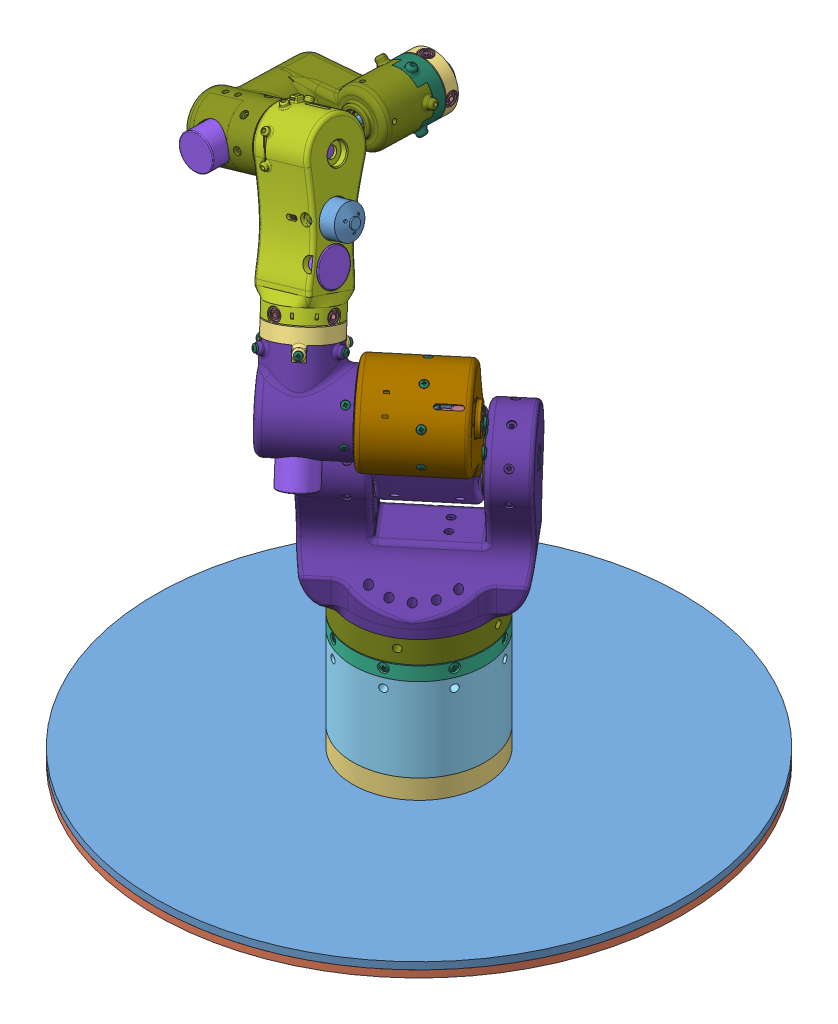
SolidWorks assembly Robotic Arm - Final Assembly, configuration Default. Lengths in mm.
Overall size (819.62 693.08 819.62).
163 component instances, 57 part files, 15 mates.
Components (placement in the parent):
- Bottom Base Assembly-1: Bottom Base Assembly [Default] at (29.9883 409.5515 787.0845) size (819.62 16 819.62)
  - Top Plate-1: Top Plate [Default] at origin size (600 8 600)
  - Bottom Plate-1: Bottom Plate [Default] at (0 -8 0) x (0.866025 0 -0.5) z (0.5 0 0.866025) size (600 8 600)
- A1 - Final Assembly-1: A1 - Final Assembly [Default] at (29.9883 417.5515 787.0845) x (0.866025 0 0.5) z (-0.5 0 0.866025) size (210.32 133.5 210.32)
  - A1D1 - Bottom-1: A1D1 - Bottom [Default] at origin size (150 22 150)
  - Turnigy Aerodrive SK3 4250-1: Turnigy Aerodrive SK3 4250 [Default] at (0 73.3 0) x (-0.707107 0 -0.707107) z (-0.707107 0 0.707107) size (52.1 79.08 41.8)
  - A1D2 - Middle-1: A1D2 - Middle [Default] at (0 22 0) x (0.991445 0 -0.130526) z (0.130526 0 0.991445) size (150 96 150)
  - A1D3 - Top-1: A1D3 - Top [Default] at (0 117 0) x (0.793353 0 0.608761) z (-0.608761 0 0.793353) size (150 15.5 150)
  - A1D4 - Encoder bracket-1: A1D4 - Encoder bracket [Default] at (0 30 0) x (0.991445 0 -0.130526) z (0.130526 0 0.991445) size (52.04 50 76.58)
  - Encoder600PR-1: Encoder600PR [Default] at (-40.4994 32.32 -24.4547) x (0.84353 0 0.537082) z (-0.537082 0 0.84353) size (38 53 38)
  - A1P1_S1 - BLDC Axis Bottom (50T HTD3m)-1: A1P1_S1 - BLDC Axis Bottom (50T HTD3m) [Default] at (-3.3955 88.2939 1.3517) x (0.767493 0 -0.641057) z (0 -1 0) size (46.98 46.92 14.7)
  - A1P1_S2 - BLDC Axis Top (Sun in A1R1)-1: A1P1_S2 - BLDC Axis Top (Sun in A1R1) [Default] at (-3.3955 88.2939 1.3517) x (0.767493 0 -0.641057) z (0 -1 0) size (38.1 38.1 28.24)
  - A1P2 - Encoder Axis (20T HTD3m)-1: A1P2 - Encoder Axis (20T HTD3m) [Default] at (-40.4994 73.3 -24.4547) x (0.825705 0 -0.564102) z (0 1 0) size (21.34 40.98 60.33)
  - radial ball bearing_68_am-3: radial ball bearing_68_am [AFBMA 20.1 - 00-70 - 18,DE,AC,18_68] at (0 126 0) x (0 1 0) z (0 0 1) size (13.2 110 110)
  - radial ball bearing_68_iso-1: radial ball bearing_68_iso [ISO 15 RBB - 105 - 8,SI,NC,8_68] at (8.4842 126.5 64.4439) x (0.130526 0 0.991445) z (-0.991445 0 0.130526) size (5 14 14)
  - radial ball bearing_68_iso-2: radial ball bearing_68_iso [ISO 15 RBB - 105 - 8,SI,NC,8_68] at (51.568 126.5 39.5695) x (0.793353 0 0.608761) z (-0.608761 0 0.793353) size (5 14 14)
  - radial ball bearing_68_iso-3: radial ball bearing_68_iso [ISO 15 RBB - 105 - 8,SI,NC,8_68] at (64.4439 126.5 -8.4842) x (0.991445 0 -0.130526) z (0.130526 0 0.991445) size (5 14 14)
  - radial ball bearing_68_iso-4: radial ball bearing_68_iso [ISO 15 RBB - 105 - 8,SI,NC,8_68] at (39.5695 126.5 -51.568) x (0.608761 0 -0.793353) z (0.793353 0 0.608761) size (5 14 14)
  - radial ball bearing_68_iso-5: radial ball bearing_68_iso [ISO 15 RBB - 105 - 8,SI,NC,8_68] at (-8.4842 126.5 -64.4439) x (-0.130526 0 -0.991445) z (0.991445 0 -0.130526) size (5 14 14)
  - radial ball bearing_68_iso-6: radial ball bearing_68_iso [ISO 15 RBB - 105 - 8,SI,NC,8_68] at (-51.568 126.5 -39.5695) x (-0.793353 0 -0.608761) z (0.608761 0 -0.793353) size (5 14 14)
  - radial ball bearing_68_iso-7: radial ball bearing_68_iso [ISO 15 RBB - 105 - 8,SI,NC,8_68] at (-64.4439 126.5 8.4842) x (-0.991445 0 0.130526) z (-0.130526 0 -0.991445) size (5 14 14)
  - radial ball bearing_68_iso-8: radial ball bearing_68_iso [ISO 15 RBB - 105 - 8,SI,NC,8_68] at (-39.5695 126.5 51.568) x (-0.608761 0 0.793353) z (-0.793353 0 -0.608761) size (5 14 14)
  - A1R1 - Fixed ring (38T)-1: A1R1 - Fixed ring (38T) [Default] at (-96.4762 151.2552 -44.9758) x (0.965926 0 0.258819) z (0 1 0) size (84.14 84.14 19.84)
  - pan head cross recess screw_iso-3: pan head cross recess screw_iso [ISO 7045 - M5 x 16 - Z - 16N] at (9.7764 126.5 74.2592) x (-0.130526 0 -0.991445) z (0.264332 -0.963804 -0.0348) size (19.63 9.5 9.5)
  - pan head cross recess screw_iso-5: pan head cross recess screw_iso [ISO 7045 - M4 x 16 - Z - 16N] at (6.8787 106.5867 52.2491) x (-0.130526 0 -0.991445) z (-0.096727 -0.995229 0.012734) size (19.02 8 8)
  - pan head cross recess screw_iso-6: pan head cross recess screw_iso [ISO 7045 - M4 x 16 - Z - 16N] at (30 128.5 51.9615) x (0 -1 0) z (0.614442 0 0.788962) size (19.02 8 8)
  - pan head cross recess screw_iso-7: pan head cross recess screw_iso [ISO 7045 - M4 x 16 - Z - 16N] at (41.8097 106.5867 32.0817) x (-0.793353 0 -0.608761) z (-0.059392 -0.995229 0.077401) size (19.02 8 8)
  - pan head cross recess screw_iso-8: pan head cross recess screw_iso [ISO 7045 - M4 x 16 - Z - 16N] at (52.2491 106.5867 -6.8787) x (-0.991445 0 0.130526) z (0.012734 -0.995229 0.096727) size (19.02 8 8)
  - pan head cross recess screw_iso-9: pan head cross recess screw_iso [ISO 7045 - M4 x 16 - Z - 16N] at (32.0817 106.5867 -41.8097) x (-0.608761 0 0.793353) z (0.077401 -0.995229 0.059392) size (19.02 8 8)
  - pan head cross recess screw_iso-10: pan head cross recess screw_iso [ISO 7045 - M4 x 16 - Z - 16N] at (-6.8787 106.5867 -52.2491) x (0.130526 0 0.991445) z (0.096727 -0.995229 -0.012734) size (19.02 8 8)
  - pan head cross recess screw_iso-11: pan head cross recess screw_iso [ISO 7045 - M4 x 16 - Z - 16N] at (-41.8097 106.5867 -32.0817) x (0.793353 0 0.608761) z (0.059392 -0.995229 -0.077401) size (19.02 8 8)
  - pan head cross recess screw_iso-12: pan head cross recess screw_iso [ISO 7045 - M4 x 16 - Z - 16N] at (-52.2491 106.5867 6.8787) x (0.991445 0 -0.130526) z (-0.012734 -0.995229 -0.096727) size (19.02 8 8)
  - pan head cross recess screw_iso-13: pan head cross recess screw_iso [ISO 7045 - M4 x 16 - Z - 16N] at (-32.0817 106.5867 41.8097) x (0.608761 0 -0.793353) z (-0.077401 -0.995229 -0.059392) size (19.02 8 8)
  - pan head cross recess screw_iso-14: pan head cross recess screw_iso [ISO 7045 - M4 x 16 - Z - 16N] at (57.9555 128.5 15.5291) x (0 -1 0) z (0.992357 0 0.123404) size (19.02 8 8)
  - pan head cross recess screw_iso-15: pan head cross recess screw_iso [ISO 7045 - M4 x 16 - Z - 16N] at (51.9615 128.5 -30) x (0 -1 0) z (0.788962 0 -0.614442) size (19.02 8 8)
  - pan head cross recess screw_iso-16: pan head cross recess screw_iso [ISO 7045 - M4 x 16 - Z - 16N] at (15.5291 128.5 -57.9555) x (0 -1 0) z (0.123404 0 -0.992357) size (19.02 8 8)
  - pan head cross recess screw_iso-17: pan head cross recess screw_iso [ISO 7045 - M4 x 16 - Z - 16N] at (-30 128.5 -51.9615) x (0 -1 0) z (-0.614442 0 -0.788962) size (19.02 8 8)
  - pan head cross recess screw_iso-18: pan head cross recess screw_iso [ISO 7045 - M4 x 16 - Z - 16N] at (-57.9555 128.5 -15.5291) x (0 -1 0) z (-0.992357 0 -0.123404) size (19.02 8 8)
  - pan head cross recess screw_iso-19: pan head cross recess screw_iso [ISO 7045 - M4 x 16 - Z - 16N] at (-51.9615 128.5 30) x (0 -1 0) z (-0.788962 0 0.614442) size (19.02 8 8)
  - pan head cross recess screw_iso-20: pan head cross recess screw_iso [ISO 7045 - M4 x 16 - Z - 16N] at (-15.5291 128.5 57.9555) x (0 -1 0) z (-0.123404 0 0.992357) size (19.02 8 8)
  - pan head cross recess screw_iso-21: pan head cross recess screw_iso [ISO 7045 - M5 x 16 - Z - 16N] at (59.4222 126.5 45.5962) x (-0.793353 0 -0.608761) z (0.162304 -0.963804 -0.211518) size (19.63 9.5 9.5)
  - pan head cross recess screw_iso-22: pan head cross recess screw_iso [ISO 7045 - M5 x 16 - Z - 16N] at (74.2592 126.5 -9.7764) x (-0.991445 0 0.130526) z (-0.0348 -0.963804 -0.264332) size (19.63 9.5 9.5)
  - pan head cross recess screw_iso-23: pan head cross recess screw_iso [ISO 7045 - M5 x 16 - Z - 16N] at (45.5962 126.5 -59.4222) x (-0.608761 0 0.793353) z (-0.211518 -0.963804 -0.162304) size (19.63 9.5 9.5)
  - pan head cross recess screw_iso-24: pan head cross recess screw_iso [ISO 7045 - M5 x 16 - Z - 16N] at (-9.7764 126.5 -74.2592) x (0.130526 0 0.991445) z (-0.264332 -0.963804 0.0348) size (19.63 9.5 9.5)
  - pan head cross recess screw_iso-25: pan head cross recess screw_iso [ISO 7045 - M5 x 16 - Z - 16N] at (-59.4222 126.5 -45.5962) x (0.793353 0 0.608761) z (-0.162304 -0.963804 0.211518) size (19.63 9.5 9.5)
  - pan head cross recess screw_iso-26: pan head cross recess screw_iso [ISO 7045 - M5 x 16 - Z - 16N] at (-74.2592 126.5 9.7764) x (0.991445 0 -0.130526) z (0.0348 -0.963804 0.264332) size (19.63 9.5 9.5)
  - pan head cross recess screw_iso-27: pan head cross recess screw_iso [ISO 7045 - M5 x 16 - Z - 16N] at (-45.5962 126.5 59.4222) x (0.608761 0 -0.793353) z (0.211518 -0.963804 0.162304) size (19.63 9.5 9.5)
  - pan head cross recess screw_iso-29: pan head cross recess screw_iso [ISO 7045 - M5 x 16 - Z - 16N] at (-75.73 69.5 20.0563) x (0.991445 0 -0.130526) z (-0.041237 0.948782 -0.313228) size (19.63 9.5 9.5)
  - pan head cross recess screw_iso-30: pan head cross recess screw_iso [ISO 7045 - M5 x 16 - Z - 16N] at (-78.3405 69.5 0.2274) x (0.991445 0 -0.130526) z (0.119155 0.408217 0.905075) size (19.63 9.5 9.5)
- A2 - Final Assembly-1: A2 - Final Assembly [Default] at (-49.7513 476.7623 907.6561) x (-0.868697 0 -0.495343) z (0.495343 0 -0.868697) size (219.53 224.2 242.26)
  - A2D1 - Bottom-1: A2D1 - Bottom [Default] at (-9.5453 74.2892 144.2387) size (150 26.12 150)
  - A2D2 - Top-1: A2D2 - Top [Default] at (-9.5453 109.2892 144.2387) x (0.347743 0 -0.93759) z (0.93759 0 0.347743) size (198.9 180.3 160.37)
  - A2D4 - Motor Bracket-1: A2D4 - Motor Bracket [Default] at (7.8419 132.7892 97.3592) x (-0.93759 0 -0.347743) z (0 -1 0) size (40 16 65)
  - A2D3 - Encoder Bracket-1: A2D3 - Encoder Bracket [Default] at (-16.8479 132.7892 163.9281) x (0.93759 0 0.347743) z (-0.347743 0 0.93759) size (40 41.5 8)
  - Turnigy Aerodrive SK3 4250-1: Turnigy Aerodrive SK3 4250 [Default] at (-9.9973 132.7892 145.4575) x (0.662976 -0.707107 0.245892) z (0.662976 0.707107 0.245892) size (52.1 79.08 41.8)
  - Encoder600PR-1: Encoder600PR [Default] at (-31.8008 132.7892 204.2444) x (0.468795 -0.866025 0.173872) z (0.811977 0.5 0.301155) size (38 53 38)
  - A2D5 - Motor To Encoder Connector-1: A2D5 - Motor To Encoder Connector [Default] at (-9.9973 132.7892 145.4575) x (0.662976 -0.707107 0.245892) z (-0.347743 0 0.93759) size (22 22 21.7)
  - A2R1 - Output Ring (36T)-1: A2R1 - Output Ring (36T) [Default] at (21.7427 110.9929 177.6385) x (0.683984 0 0.729497) z (0 1 0) size (82 82 36.22)
  - A2R2 - Fixed Ring (38T)-1: A2R2 - Fixed Ring (38T) [Default] at (6.8682 231.7999 101.2643) x (0.93759 0 0.347743) z (0.347743 0 -0.93759) size (77.7 77.7 19)
  - A2R2 - Fixed Ring (38T)-3: A2R2 - Fixed Ring (38T) [Default] at (-33.609 231.7999 207.84) x (-0.93759 0 -0.347743) z (-0.347743 0 0.93759) size (77.7 77.7 19)
  - radial ball bearing_68_iso-1: radial ball bearing_68_iso [ISO 15 RBB - 1860 - 32,SI,NC,32_68] at (4.0167 231.7892 107.6727) x (0.347743 0 -0.93759) z (0.369105 -0.91925 0.136897) size (10 78 78)
  - radial ball bearing_68_iso-2: radial ball bearing_68_iso [ISO 15 RBB - 1860 - 32,SI,NC,32_68] at (-30.7576 231.7892 201.4317) x (-0.347743 0 0.93759) z (-0.369105 0.91925 -0.136897) size (10 78 78)
  - radial ball bearing_68_din-1: radial ball bearing_68_din [DIN 625 - 608 - 8,DE,NC,8_68] at (22.9687 231.7892 56.574) x (0.347743 0 -0.93759) z (-0.181317 0.981123 -0.067249) size (7 22 22)
  - radial ball bearing_68_din-2: radial ball bearing_68_din [DIN 625 - 608 - 8,DE,NC,8_68] at (-42.0593 231.7892 231.9033) x (0.347743 0 -0.93759) z (0.862216 -0.392835 0.319788) size (7 22 22)
  - A2D8 Axis D8 220mm-1: A2D8 Axis D8 220mm [Default] at (24.1858 231.7892 53.2925) x (0.915947 -0.213623 0.339716) z (-0.347743 0 0.93759) size (8 8 194)
  - A2P1 - Motor and Axis-1: A2P1 - Motor and Axis [Default] at (17.5787 132.7892 71.1067) x (0.879075 0.347743 0.326041) z (0.326041 -0.93759 0.120925) size (21 22 21)
  - A2P1 - Motor and Axis-2: A2P1 - Motor and Axis [Default] at (12.7103 231.7892 84.2329) x (-0.937346 -0.02278 -0.347653) z (0.021358 -0.999741 0.007921) size (21 22 21)
- A3 - Final Assembly-1: A3 - Final Assembly [Default] at (19.335 680.5082 758.7988) x (-0.766512 0 0.64223) z (-0.450257 0.713079 -0.537389) size (116.5 270 98)
  - A3D1 - Bottom-1: A3D1 - Bottom [Default] at origin size (99.9 135 87.01)
  - A3D2 - Top-1: A3D2 - Top [Default] at (-94.5 331 0) x (0 1 0) z (-1 0 0) size (160 98 100.36)
  - A3D3 - Motor Assembly-1: A3D3 - Motor Assembly [Default] at (-19.5 149 0) x (0 0 1) z (0 -1 0) size (46 63 103.52)
  - Turnigy Aerodrive SK3 4250-1: Turnigy Aerodrive SK3 4250 [Default] at (31.8 149 0) x (0 -0.575127 0.818064) z (0 -0.818064 -0.575127) size (52.1 79.08 41.8)
  - Encoder600PR-1: Encoder600PR [Default] at (-19.5 107 0) x (0 -0.866025 0.5) z (0 0.5 0.866025) size (38 53 38)
  - A3D8 - Motor Assembly Gear 1-1: A3D8 - Motor Assembly Gear 1 [Default] at (71.5096 132.326 18.6577) x (1 0 0) z (0 0.420901 0.907106) size (4 42.98 42.98)
  - A3D9 - Motor Assembly Gear 2-1: A3D9 - Motor Assembly Gear 2 [Default] at (-13.5987 96.6456 14.6355) x (-1 0 0) z (0 -0.921751 -0.387782) size (15 43.41 43.41)
  - Pulley HTD_3mm T20 D5-1: Pulley HTD_3mm T20 D5 [Default] at (-41.5 149 0) x (0 -0.987714 0.156271) z (0 0.156271 0.987714) size (21 22 21)
  - A3D4 - Output Ring-1: A3D4 - Output Ring [Default] at (1.3 221.0108 0.045) x (0 0 -1) z (-1 0 0) size (76.49 77.19 18.96)
  - radial ball bearing_68_iso-1: radial ball bearing_68_iso [ISO 15 RBB - 1860 - 32,SI,NC,32_68] at (8.8 221 0) size (10 78 78)
  - radial ball bearing_68_iso-2: radial ball bearing_68_iso [ISO 15 RBB - 1860 - 32,SI,NC,32_68] at (42.5 221 0) x (1 0 0) z (0 -0.007607 0.999971) size (10 78 78)
  - Axis D8 197mm-1: Axis D8 197mm [Default] at (-52.5 221 0) x (0 0 -1) z (1 0 0) size (8 8 114)
  - radial ball bearing_68_din-1: radial ball bearing_68_din [DIN 625 - 608 - 8,DE,NC,8_68] at (-49 221 0) x (-1 0 0) z (0 -0.924225 -0.381849) size (7 22 22)
  - Pulley HTD_3mm T20 D5-3: Pulley HTD_3mm T20 D5 [Default] at (-41.5 221 0) x (0 0.38968 0.92095) z (0 0.92095 -0.38968) size (21 22 21)
  - A3D5 - Input Ring-1: A3D5 - Input Ring [Default] at (53.8 40 0) x (0 0 -1) z (1 0 0) size (65.4 65.4 34.7)
  - A3D5 - Input Ring-2: A3D5 - Input Ring [Default] at (-53.8 40 0) x (0 0 1) z (-1 0 0) size (65.4 65.4 34.7)
  - pan head cross recess screw_iso-3: pan head cross recess screw_iso [ISO 7045 - M4 x 16 - Z - 16N] at (-26.3 53.202 -36.2721) x (0 -0.34202 0.939693) z (-0.509751 -0.808438 -0.294247) size (19.02 8 8)
  - pan head cross recess screw_iso-4: pan head cross recess screw_iso [ISO 7045 - M4 x 16 - Z - 16N] at (-26.3 17.8599 -31.6193) x (0 0.573576 0.819152) z (-0.509751 -0.704734 0.49346) size (19.02 8 8)
  - pan head cross recess screw_iso-5: pan head cross recess screw_iso [ISO 7045 - M4 x 16 - Z - 16N] at (-26.3 1.4 0) x (0 1 0) z (-0.509751 0 0.860322) size (19.02 8 8)
  - pan head cross recess screw_iso-6: pan head cross recess screw_iso [ISO 7045 - M4 x 16 - Z - 16N] at (-26.3 17.8599 31.6193) x (0 0.573576 -0.819152) z (-0.509751 0.704734 0.49346) size (19.02 8 8)
  - pan head cross recess screw_iso-7: pan head cross recess screw_iso [ISO 7045 - M4 x 16 - Z - 16N] at (-26.3 53.202 36.2721) x (0 -0.34202 -0.939693) z (-0.509751 0.808438 -0.294247) size (19.02 8 8)
  - pan head cross recess screw_iso-12: pan head cross recess screw_iso [ISO 7045 - M4 x 16 - Z - 16N] at (26.2 53.202 36.2721) x (0 -0.34202 -0.939693) z (-0.509751 0.808438 -0.294247) size (19.02 8 8)
  - pan head cross recess screw_iso-13: pan head cross recess screw_iso [ISO 7045 - M4 x 16 - Z - 16N] at (26.2 17.8599 31.6193) x (0 0.573576 -0.819152) z (-0.509751 0.704734 0.49346) size (19.02 8 8)
  - pan head cross recess screw_iso-14: pan head cross recess screw_iso [ISO 7045 - M4 x 16 - Z - 16N] at (26.2 1.4 0) x (0 1 0) z (-0.509751 0 0.860322) size (19.02 8 8)
  - pan head cross recess screw_iso-15: pan head cross recess screw_iso [ISO 7045 - M4 x 16 - Z - 16N] at (26.2 17.8599 -31.6193) x (0 0.573576 0.819152) z (-0.509751 -0.704734 0.49346) size (19.02 8 8)
  - pan head cross recess screw_iso-16: pan head cross recess screw_iso [ISO 7045 - M4 x 16 - Z - 16N] at (26.2 53.202 -36.2721) x (0 -0.34202 0.939693) z (-0.509751 -0.808438 -0.294247) size (19.02 8 8)
  - pan head cross recess screw_iso-17: pan head cross recess screw_iso [ISO 7045 - M4 x 16 - Z - 16N] at (-7.2 201.8276 -46.2864) x (0 0.382683 0.92388) z (-0.246103 -0.895464 0.370913) size (19.02 8 8)
  - pan head cross recess screw_iso-18: pan head cross recess screw_iso [ISO 7045 - M4 x 16 - Z - 16N] at (-7.2 240.1724 -46.2864) x (0 -0.382683 0.92388) z (-0.246103 -0.895464 -0.370913) size (19.02 8 8)
  - pan head cross recess screw_iso-19: pan head cross recess screw_iso [ISO 7045 - M4 x 16 - Z - 16N] at (-7.2 267.2864 -19.1724) x (0 -0.92388 0.382683) z (-0.246103 -0.370913 -0.895464) size (19.02 8 8)
  - pan head cross recess screw_iso-20: pan head cross recess screw_iso [ISO 7045 - M4 x 16 - Z - 16N] at (-7.2 267.2864 19.1724) x (0 -0.92388 -0.382683) z (-0.246103 0.370913 -0.895464) size (19.02 8 8)
  - pan head cross recess screw_iso-21: pan head cross recess screw_iso [ISO 7045 - M4 x 16 - Z - 16N] at (-7.2 240.1724 46.2864) x (0 -0.382683 -0.92388) z (-0.246103 0.895464 -0.370913) size (19.02 8 8)
  - pan head cross recess screw_iso-22: pan head cross recess screw_iso [ISO 7045 - M4 x 16 - Z - 16N] at (-7.2 201.8276 46.2864) x (0 0.382683 -0.92388) z (-0.246103 0.895464 0.370913) size (19.02 8 8)
  - pan head cross recess screw_iso-23: pan head cross recess screw_iso [ISO 7045 - M4 x 16 - Z - 16N] at (50.6 128 14) x (-1 0 0) z (0 -0.78047 0.625193) size (19.02 8 8)
  - pan head cross recess screw_iso-24: pan head cross recess screw_iso [ISO 7045 - M4 x 16 - Z - 16N] at (50.6 128 -14) x (-1 0 0) z (0 -0.872039 0.489436) size (19.02 8 8)
  - pan head cross recess screw_iso-25: pan head cross recess screw_iso [ISO 7045 - M4 x 16 - Z - 16N] at (-6.6 178.2028 10) x (-1 0 0) z (0 -0.78047 0.625193) size (19.02 8 8)
  - pan head cross recess screw_iso-26: pan head cross recess screw_iso [ISO 7045 - M4 x 16 - Z - 16N] at (-6.6 178.2028 -10) x (-1 0 0) z (0 -0.857112 0.51513) size (19.02 8 8)
  - pan head cross recess screw_iso-28: pan head cross recess screw_iso [ISO 7045 - M5 x 20 - Z - 20N] at (-51.2 129.5 12) size (23.63 9.5 9.5)
  - pan head cross recess screw_iso-30: pan head cross recess screw_iso [ISO 7045 - M5 x 20 - Z - 20N] at (-51.2 129.5 -12) size (23.63 9.5 9.5)
  - pan head cross recess screw_iso-31: pan head cross recess screw_iso [ISO 7045 - M5 x 20 - Z - 20N] at (-48.9707 102 10) x (1 0 0) z (0 -0.0226 0.999745) size (23.63 9.5 9.5)
  - pan head cross recess screw_iso-32: pan head cross recess screw_iso [ISO 7045 - M5 x 20 - Z - 20N] at (-49.1838 102 -10) x (1 0 0) z (0 0.345979 0.938242) size (23.63 9.5 9.5)
- A4 Assembly-1: A4 Assembly [Default] at (62.4341 798.6751 948.818) x (-0.766512 0 0.64223) z (-0.59041 -0.393527 -0.704665) size (141.2 141.04 102.76)
  - A4D1 - Main-1: A4D1 - Main [Default] at origin size (84.74 100.7 81.3)
  - Encoder600PR-1: Encoder600PR [Default] at (5.5 -25.7 0) x (-0.74134 0 0.67113) z (-0.67113 0 -0.74134) size (38 53 38)
  - A4D3 - Spacer-1: A4D3 - Spacer [Default] at (-51.5 40 0) x (0 0.966883 -0.25522) z (0 0.25522 0.966883) size (77 33.7 77)
  - Propdrive v2 3536-910kv-1: Propdrive v2 3536-910kv [Default] at (5.5 35 0) size (35.77 56 35.77)
  - A4D4 - Output-1: A4D4 - Output [Default] at (-66.3918 137.7518 -78.5095) x (0.793353 0 0.608761) z (0 1 0) size (61.85 61.85 14.17)
  - A4D5 - Output connector-1: A4D5 - Output connector [Default] at (5.5 85.9983 0) x (-0.5 0 -0.866025) z (0.866025 0 -0.5) size (74.78 29.34 76)
  - radial ball bearing_68_am-1: radial ball bearing_68_am [AFBMA 20.1 - 17-50 - 40,DE,NC,40_68] at (5.5 108.6683 0) x (0 1 0) z (0.187116 0 0.982338) size (6 62 62)
  - Propdrive v2 3536-910kv Aidpiece-1: Propdrive v2 3536-910kv Aidpiece [Default] at (5.5 37 0) x (0.832034 0 -0.554724) z (0 -1 0) size (22 22 21.7)
  - pan head cross recess screw_iso-2: pan head cross recess screw_iso [ISO 7045 - M4 x 16 - Z - 16N] at (-33.5 53.7274 -37.7158) x (0 -0.34202 0.939693) z (-0.938857 0.323544 0.11776) size (19.02 8 8)
  - pan head cross recess screw_iso-3: pan head cross recess screw_iso [ISO 7045 - M4 x 16 - Z - 16N] at (-33.5 53.76 37.8052) x (0 -0.34202 -0.939693) z (0.961212 -0.259176 0.094332) size (19.02 8 8)
  - pan head cross recess screw_iso-4: pan head cross recess screw_iso [ISO 7045 - M4 x 16 - Z - 16N] at (-33.5 16.9623 32.9012) x (0 0.573576 -0.819152) z (0.822308 0.466132 0.326389) size (19.02 8 8)
  - pan head cross recess screw_iso-5: pan head cross recess screw_iso [ISO 7045 - M4 x 16 - Z - 16N] at (-33.5 -0.1713 0) x (0 1 0) z (-0.025418 0 0.999677) size (19.02 8 8)
  - pan head cross recess screw_iso-6: pan head cross recess screw_iso [ISO 7045 - M4 x 16 - Z - 16N] at (-33.5 16.9893 -32.8627) x (0 0.573576 0.819152) z (-0.783337 -0.509183 0.356534) size (19.02 8 8)
  - pan head cross recess screw_iso-8: pan head cross recess screw_iso [ISO 7045 - M4 x 16 - Z - 16N] at (43.9515 93.085 -22.2) x (-0.866025 0 0.5) z (-0.5 0 -0.866025) size (19.02 8 8)
  - pan head cross recess screw_iso-9: pan head cross recess screw_iso [ISO 7045 - M4 x 16 - Z - 16N] at (-32.6917 93.0833 22.05) x (0.866025 0 -0.5) z (0.5 0 0.866025) size (19.02 8 8)
  - pan head cross recess screw_iso-10: pan head cross recess screw_iso [ISO 7045 - M4 x 16 - Z - 16N] at (5.5 93.0833 -44.1) x (0 0 1) z (-1 0 0) size (19.02 8 8)
  - pan head cross recess screw_iso-11: pan head cross recess screw_iso [ISO 7045 - M4 x 16 - Z - 16N] at (5.5 93.085 44.4) x (0 0 -1) z (1 0 0) size (19.02 8 8)
  - pan head cross recess screw_iso-12: pan head cross recess screw_iso [ISO 7045 - M4 x 16 - Z - 16N] at (43.6917 93.0833 22.05) x (-0.866025 0 -0.5) z (0.5 0 -0.866025) size (19.02 8 8)
  - pan head cross recess screw_iso-13: pan head cross recess screw_iso [ISO 7045 - M4 x 16 - Z - 16N] at (-32.9515 93.085 -22.2) x (0.866025 0 0.5) z (-0.5 0 0.866025) size (19.02 8 8)
  - A4D2 - Input from A3 (alt-50)-1: A4D2 - Input from A3 (alt-50) [Default] at (-85 40 0) x (0 0 1) z (-1 0 0) size (65.4 65.4 59.2)
- A5 Assembly-1: A5 Assembly [Default] at (93.5083 918.5196 932.5261) x (0.5396 0.392703 0.744726) z (-0.252735 0.919313 -0.301643) size (117.85 116.54 195.47)
  - A5D1 - Input Ring-3: A5D1 - Input Ring [Default] at (-5.5765 -43.1726 42.7362) size (53.6 53.6 26.97)
  - Encoder600PR-2: Encoder600PR [Default] at (-32.2392 -16.8999 55.5428) x (0.809017 -0.587785 -0.000664) z (-0.000537 0.000391 -1) size (38 53 38)
  - A5D2 - Main-2: A5D2 - Main [Default] at (-51.3422 -43.193 34.1028) x (0.587785 0.809017 0) z (0.809017 -0.587785 0) size (80.94 180.44 86.87)
  - Propdrive v2 3536-910kv-2: Propdrive v2 3536-910kv [Default] at (-19.21 1.0333 95.5428) x (0.576802 -0.419071 -0.701198) z (-0.567281 0.412154 -0.712967) size (35.77 56 35.77)
  - Pulley HTD_3mm T60 D8-1: Pulley HTD_3mm T60 D8 [Default] at (-56.0759 -49.7083 149.1028) x (-0.142543 0.103564 -0.984356) z (0.79636 -0.57859 -0.176193) size (60 25 60)
  - radial ball bearing_68_am-1: radial ball bearing_68_am [AFBMA 20.1 - 17-50 - 40,DE,NC,40_68] at (-68.0941 -66.25 149.1028) x (0.587785 0.809017 0) z (-0.798405 0.580075 -0.161441) size (6 62 62) (hidden)
  - A5D7 - Encoder Sun-1: A5D7 - Encoder Sun [Default] at (-53.2293 -54.7697 50.8784) x (0.72854 -0.529315 0.434804) z (-0.587785 -0.809017 0) size (17 16.93 18)
  - A5D3 - Output Ring-1: A5D3 - Output Ring [Default] at (-64.8511 -62.4299 149.1136) x (0.809017 -0.587785 0) z (0.587785 0.809017 0) size (60.74 61.32 16.45)
  - radial ball bearing_68_din-1: radial ball bearing_68_din [DIN 625 - 608 - 8,DE,NC,8_68] at (-71.9147 -71.5086 95.5428) x (-0.587785 -0.809017 0) z (0.370529 -0.269205 0.888953) size (7 22 22)
  - radial ball bearing_68_iso-1: radial ball bearing_68_iso [ISO 15 RBB - 105 - 8,SI,NC,8_68] at (-69.5636 -68.2725 15.1028) x (-0.587785 -0.809017 0) z (-0.658083 0.478125 0.581656) size (5 14 14)
  - radial ball bearing_68_iso-2: radial ball bearing_68_iso [ISO 15 RBB - 105 - 8,SI,NC,8_68] at (-26.2627 -61.4143 15.1028) x (0.809017 -0.587785 0) z (-0.478125 -0.658083 0.581656) size (5 14 14)
  - radial ball bearing_68_iso-3: radial ball bearing_68_iso [ISO 15 RBB - 105 - 8,SI,NC,8_68] at (-33.1209 -18.1135 15.1028) x (0.587785 0.809017 0) z (0.658083 -0.478125 0.581656) size (5 14 14)
  - radial ball bearing_68_iso-4: radial ball bearing_68_iso [ISO 15 RBB - 105 - 8,SI,NC,8_68] at (-76.4218 -24.9717 15.1028) x (-0.809017 0.587785 0) z (0.478125 0.658083 0.581656) size (5 14 14)
  - A5D5 - BLDC Sun-1: A5D5 - BLDC Sun [Default] at (-43.3092 -32.1364 95.5428) x (0.221765 -0.161121 -0.961697) z (-0.587785 -0.809017 0) size (24 24 50.67)
  - A5D6 - Axis holder-2: A5D6 - Axis holder [Default] at (-67.5063 -65.441 95.5428) x (-0.572061 0.415627 -0.707107) z (-0.572061 0.415627 0.707107) size (49 11 49)
  - Bearing - I50 - O62 - D6-1: Bearing - I50 - O62 - D6 [AFBMA 20.1 - 17-50 - 40,DE,NC,40_68] at (-68.0961 -66.2527 149.1028) x (0.587785 0.809017 0) z (-0.219405 0.159407 0.962523) size (6 62 62)
- A6 Assembly-1: A6 Assembly [Default] at (-76.4768 983.4828 968.382) x (0.966884 0.251416 -0.043878) z (-0.253404 0.966175 -0.047874) size (157.9 177.54 88.85)
  - Encoder600PR-1: Encoder600PR [Default] at (3.921 38.6161 35.8814) x (0.31767 0 -0.948201) z (0.948201 0 0.31767) size (38 53 38)
  - Propdrive v2 3536-910kv-1: Propdrive v2 3536-910kv [Default] at (3.921 99.3161 35.8814) x (0.262612 0 -0.964901) z (0.964901 0 0.262612) size (35.77 56 35.77)
  - A6D2 - Output Ring-1: A6D2 - Output Ring [Default] at (62.5859 241.5311 -68.312) x (0.372467 0 0.928046) z (0 1 0) size (51.9 51.9 11.34)
  - A6D3 - Output Bracket-1: A6D3 - Output Bracket [Default] at (84.421 191.1961 35.8814) x (0.866025 0 0.5) z (-0.5 0 0.866025) size (62.86 29.34 66.3)
  - radial ball bearing_68_iso-6: radial ball bearing_68_iso [ISO 15 RBB - 1840 - 32,SI,NC,32_68] at (84.421 209.6561 35.8814) x (0 1 0) z (-0.843815 0 0.536635) size (7 52 52)
  - A6D1 - Main-1: A6D1 - Main [Default] at (12.946 55.6161 35.8814) x (-1 0 0) z (0 0 -1) size (149.14 147.19 68.51)
  - A6 - Input Ring (alt-50)-1: A6 - Input Ring (alt-50) [Default] at (60.2543 88.1161 35.8814) x (0 0 -1) z (1 0 0) size (52 52 32.37)
  - pulley_24T-1: pulley_24T [Default] at (3.921 174.3161 35.8814) x (0.675233 0 -0.737605) z (0 -1 0) size (25.16 25.16 56)
  - pulley_24T_receiver-1: pulley_24T_receiver [Default] at (84.421 159.3161 35.8814) x (-0.910803 0 -0.412841) z (0 1 0) size (25.16 25.16 61.72)
- End Assembly-1: End Assembly [Default] at (-10.6938 1001.6639 810.582) x (-0.587621 -0.806579 0.064278) z (-0.030357 -0.057407 -0.997889) size (83.81 83.81 30.01)
  - End - Input Ring-1: End - Input Ring [Default] at (21.1766 15.3608 95.6965) size (43.6 43.6 25.5)
  - radial ball bearing_68_iso-2: radial ball bearing_68_iso [ISO 15 RBB - 105 - 8,SI,NC,8_68] at (-46.8371 31.484 68.7298) x (-0.809017 0.587785 0) z (0 0 1) size (5 14 14)
  - radial ball bearing_68_iso-3: radial ball bearing_68_iso [ISO 15 RBB - 105 - 8,SI,NC,8_68] at (-40.7532 -6.928 68.7298) x (-0.587785 -0.809017 0) z (0 0 1) size (5 14 14)
  - radial ball bearing_68_iso-4: radial ball bearing_68_iso [ISO 15 RBB - 105 - 8,SI,NC,8_68] at (-2.3412 -0.8441 68.7298) x (0.809017 -0.587785 0) z (0 0 1) size (5 14 14)
  - radial ball bearing_68_iso-5: radial ball bearing_68_iso [ISO 15 RBB - 105 - 8,SI,NC,8_68] at (-8.4251 37.5679 68.7298) x (0.587785 0.809017 0) z (0 0 1) size (5 14 14)
  - End D2 - Cap-1: End D2 - Cap [Default] at (-24.5892 15.32 62.7298) x (0.809017 -0.587785 0) z (-0.587785 -0.809017 0) size (60 16.45 60)
Mates (geometry in assembly coordinates):
- Concentric1: concentric anti-aligned: cylinder of Bottom Base Assembly-1/Top Plate-1 through (-21.9733 417.5515 757.0845) axis (0 -1 0) radius 2.05; cylinder of A1 - Final Assembly-1/A1D1 - Bottom-1 through (-21.9733 393.8098 757.0845) axis (0 1 0) radius 2.05
- Concentric2: concentric anti-aligned: cylinder of Bottom Base Assembly-1/Top Plate-1 through (-0.0117 417.5515 839.046) axis (0 -1 0) radius 2.05; cylinder of A1 - Final Assembly-1/A1D1 - Bottom-1 through (-0.0117 393.8098 839.046) axis (0 1 0) radius 2.05
- Coincident1: coincident anti-aligned: plane of Bottom Base Assembly-1/Top Plate-1 through (29.9883 417.5515 787.0845) normal (0 1 0); plane of A1 - Final Assembly-1/A1D1 - Bottom-1 through (29.9883 417.5515 787.0845) normal (0 -1 0)
- Concentric3: concentric aligned: cylinder of A1 - Final Assembly-1/radial ball bearing_68_am-3 through (29.9883 522.914 787.0845) axis (0 1 0) radius 35; cylinder of A2 - Final Assembly-1/A2R1 - Output Ring (36T)-1 through (29.9883 433.459 787.0845) axis (0 1 0) radius 35.1
- Tangent1: tangent anti-aligned: cylinder of A1 - Final Assembly-1/radial ball bearing_68_iso-6 through (13.0115 544.0515 746.0989) axis (-0.382683 0 -0.92388) radius 7; plane of A2 - Final Assembly-1/A2D1 - Bottom-1 through (67.139 551.0515 721.9322) normal (0 -1 0)
- Concentric4: concentric anti-aligned: cylinder of A2 - Final Assembly-1/A2D8 Axis D8 220mm-1 through (104.34 708.5515 724.7882) axis (-0.766512 0 0.64223) radius 4; circle of A3 - Final Assembly-1/A3D1 - Bottom-1
- Coincident2: coincident anti-aligned: plane of A2 - Final Assembly-1/radial ball bearing_68_iso-1 through (-17.5036 722.8419 783.3427) normal (0.766512 0 -0.64223); plane of A3 - Final Assembly-1/A3D1 - Bottom-1 through (3.9268 708.5515 808.9203) normal (-0.766512 0 0.64223)
- Concentric5: concentric aligned: cylinder of A3 - Final Assembly-1/radial ball bearing_68_iso-2 through (103.7864 835.4476 893.6346) axis (-0.766512 0 0.64223) radius 30; cylinder of A4 Assembly-1/A4D3 - Spacer-1 through (117.6315 835.4476 882.0344) axis (-0.766512 0 0.64223) radius 32.7
- Coincident3: coincident anti-aligned: plane of A3 - Final Assembly-1/radial ball bearing_68_iso-2 through (97.907 856.8542 926.5369) normal (-0.766512 0 0.64223); plane of A4 Assembly-1/A4D1 - Main-1 through (84.1349 835.4476 910.0998) normal (0.766512 0 -0.64223)
- Concentric6: concentric aligned: cylinder of A4 Assembly-1/radial ball bearing_68_am-1 through (35.9698 879.603 925.7964) axis (-0.252735 0.919313 -0.301643) radius 25; cylinder of A5 Assembly-1/A5D1 - Input Ring-3 through (51.1157 824.5105 943.8732) axis (-0.252735 0.919313 -0.301643) radius 25.06
- Tangent2: tangent anti-aligned: plane of A4 Assembly-1/A4D5 - Output connector-1 through (29.0683 904.7071 917.5593) normal (-0.252735 0.919313 -0.301643); cylinder of A5 Assembly-1/radial ball bearing_68_iso-2 through (26.9312 914.2795 925.3172) axis (-0.0355 0.302743 0.952411) radius 7
- Concentric7: concentric aligned: cylinder of A5 Assembly-1/A5D2 - Main-2 through (-40.4177 1025.5283 876.5638) axis (0.966884 0.251416 -0.043878) radius 30.95; cylinder of A6 Assembly-1/A6 - Input Ring (alt-50)-1 through (-45.0525 1024.3231 876.7741) axis (0.966884 0.251416 -0.043878) radius 25.1
- Coincident7: coincident anti-aligned: plane of A5 Assembly-1/Bearing - I50 - O62 - D6-1 through (-34.0282 1010.621 852.0305) normal (-0.966884 -0.251416 0.043878); plane of A6 Assembly-1/A6D1 - Main-1 through (-37.0274 1026.4098 876.4099) normal (0.966884 0.251416 -0.043878)
- Concentric8: concentric aligned: cylinder of A6 Assembly-1/radial ball bearing_68_iso-6 through (-9.682 1028.5243 774.3405) axis (-0.030357 -0.057407 -0.997889) radius 20; cylinder of End Assembly-1/End - Input Ring-1 through (-8.3296 1031.0819 818.7972) axis (-0.030357 -0.057407 -0.997889) radius 20.1
- Coincident8: coincident anti-aligned: plane of A6 Assembly-1/radial ball bearing_68_iso-6 through (-17.5842 1004.5459 758.7865) normal (0.030357 0.057407 0.997889); plane of End Assembly-1/End - Input Ring-1 through (-10.2022 1027.5405 757.2391) normal (-0.030357 -0.057407 -0.997889)
